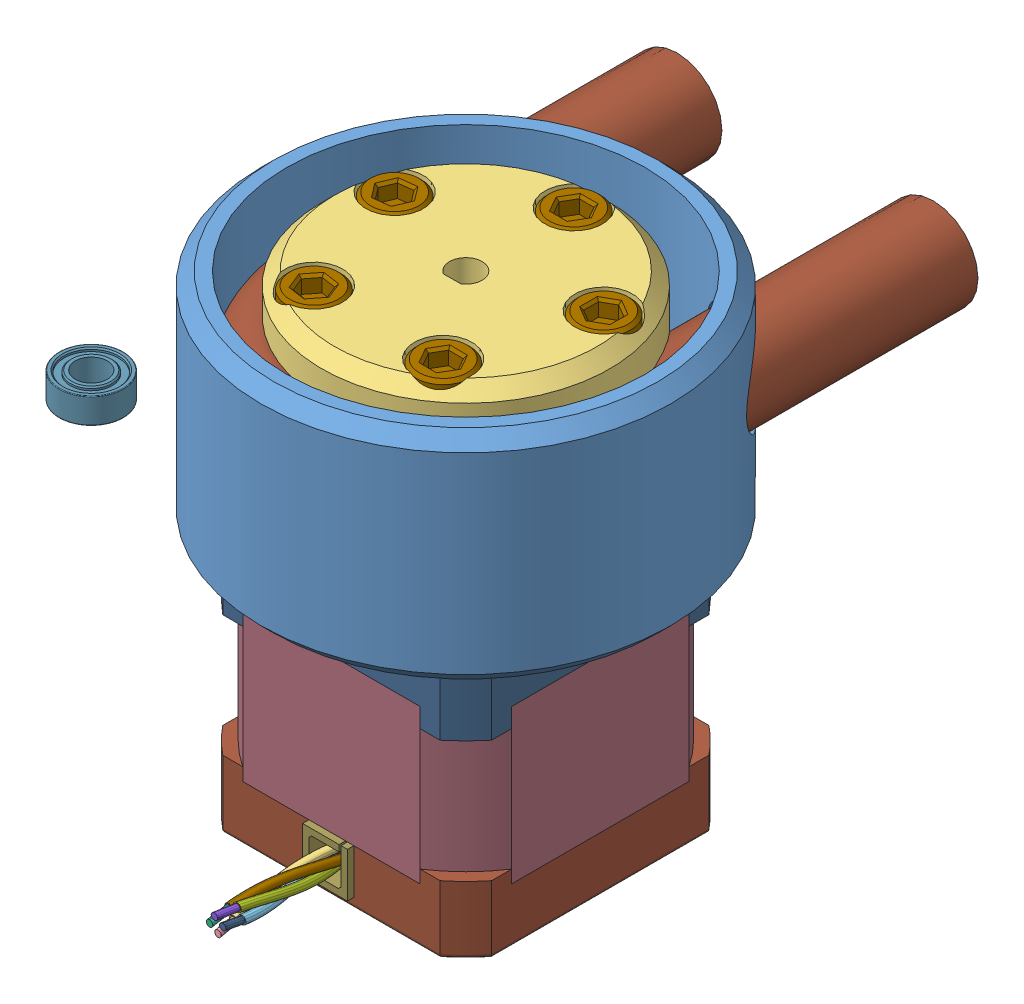
SolidWorks assembly pump, configuration Default. Lengths in mm.
Overall size (68.76 74.29 92).
175 component instances, 32 part files, 74 mates.
Components (placement in the parent):
- pump-shell-1: pump-shell [Default] at (23.8184 9.0777 41.5855) size (64 34 64)
- bottom-plate-1: bottom-plate [Default] at (23.8184 23.0777 41.5855) x (-0.999957 0 0.009262) z (0.009262 0 0.999957) size (52 18 52)
- top-plate-1: top-plate [Default] at (23.8184 35.0777 41.5855) x (-0.814427 0 -0.580267) z (0.580267 0 -0.814427) size (45 8.29 45)
- 625zz.STEP-1: 625zz.STEP [Default] at (23.8184 16.0777 41.5855) x (0 -1 0) z (-0.839089 0 -0.543994) size (5 16 16)
  - SKF 625 Inner Race^SKF 625.STEP-1: SKF 625 Inner Race^SKF 625.STEP [Default] at origin size (5 8.4 8.4)
  - SKF 625 Outer Race^SKF 625.STEP-1: SKF 625 Outer Race^SKF 625.STEP [Default] at origin size (5 16 16)
  - SKF 625 Ball^SKF 625.STEP-1: SKF 625 Ball^SKF 625.STEP [Default] at origin size (2.38 2.38 2.38)
  - SKF 625 Ball^SKF 625.STEP-2: SKF 625 Ball^SKF 625.STEP [Default] x (1 0 0) z (0 0.707107 0.707107) size (2.38 2.38 2.38)
  - SKF 625 Ball^SKF 625.STEP-3: SKF 625 Ball^SKF 625.STEP [Default] x (1 0 0) z (0 1 0) size (2.38 2.38 2.38)
  - SKF 625 Ball^SKF 625.STEP-4: SKF 625 Ball^SKF 625.STEP [Default] x (1 0 0) z (0 0.707107 -0.707107) size (2.38 2.38 2.38)
  - SKF 625 Ball^SKF 625.STEP-5: SKF 625 Ball^SKF 625.STEP [Default] x (1 0 0) z (0 0 -1) size (2.38 2.38 2.38)
  - SKF 625 Ball^SKF 625.STEP-6: SKF 625 Ball^SKF 625.STEP [Default] x (1 0 0) z (0 -0.707107 -0.707107) size (2.38 2.38 2.38)
  - SKF 625 Ball^SKF 625.STEP-7: SKF 625 Ball^SKF 625.STEP [Default] x (1 0 0) z (0 -1 0) size (2.38 2.38 2.38)
  - SKF 625 Ball^SKF 625.STEP-8: SKF 625 Ball^SKF 625.STEP [Default] x (1 0 0) z (0 -0.707107 0.707107) size (2.38 2.38 2.38)
  - SKF 625 Cage^SKF 625.STEP-1: SKF 625 Cage^SKF 625.STEP [Default] at (2.5 0 0) x (0 0 -1) z (1 0 0) size (12.17 12.17 2.88)
- m5-spacer-1: m5-spacer [Default] at (23.8184 16.0777 41.5855) x (-0.754389 0 0.656427) z (-0.656427 0 -0.754389) size (10 1 10)
- 625zz.STEP-2: 625zz.STEP [Default] at (7.5901 29.0777 36.4783) x (0 -1 0) z (0 0 1) size (5 16 16)
  - SKF 625 Inner Race^SKF 625.STEP-1: SKF 625 Inner Race^SKF 625.STEP [Default] at origin size (5 8.4 8.4)
  - SKF 625 Outer Race^SKF 625.STEP-1: SKF 625 Outer Race^SKF 625.STEP [Default] at origin size (5 16 16)
  - SKF 625 Ball^SKF 625.STEP-1: SKF 625 Ball^SKF 625.STEP [Default] at origin size (2.38 2.38 2.38)
  - SKF 625 Ball^SKF 625.STEP-2: SKF 625 Ball^SKF 625.STEP [Default] x (1 0 0) z (0 0.707107 0.707107) size (2.38 2.38 2.38)
  - SKF 625 Ball^SKF 625.STEP-3: SKF 625 Ball^SKF 625.STEP [Default] x (1 0 0) z (0 1 0) size (2.38 2.38 2.38)
  - SKF 625 Ball^SKF 625.STEP-4: SKF 625 Ball^SKF 625.STEP [Default] x (1 0 0) z (0 0.707107 -0.707107) size (2.38 2.38 2.38)
  - SKF 625 Ball^SKF 625.STEP-5: SKF 625 Ball^SKF 625.STEP [Default] x (1 0 0) z (0 0 -1) size (2.38 2.38 2.38)
  - SKF 625 Ball^SKF 625.STEP-6: SKF 625 Ball^SKF 625.STEP [Default] x (1 0 0) z (0 -0.707107 -0.707107) size (2.38 2.38 2.38)
  - SKF 625 Ball^SKF 625.STEP-7: SKF 625 Ball^SKF 625.STEP [Default] x (1 0 0) z (0 -1 0) size (2.38 2.38 2.38)
  - SKF 625 Ball^SKF 625.STEP-8: SKF 625 Ball^SKF 625.STEP [Default] x (1 0 0) z (0 -0.707107 0.707107) size (2.38 2.38 2.38)
  - SKF 625 Cage^SKF 625.STEP-1: SKF 625 Cage^SKF 625.STEP [Default] at (2.5 0 0) x (0 0 -1) z (1 0 0) size (12.17 12.17 2.88)
- 625zz.STEP-3: 625zz.STEP [Default] at (7.5901 34.0777 36.4783) x (0 -1 0) z (0.968021 0 0.25087) size (5 16 16)
  - SKF 625 Inner Race^SKF 625.STEP-1: SKF 625 Inner Race^SKF 625.STEP [Default] at origin size (5 8.4 8.4)
  - SKF 625 Outer Race^SKF 625.STEP-1: SKF 625 Outer Race^SKF 625.STEP [Default] at origin size (5 16 16)
  - SKF 625 Ball^SKF 625.STEP-1: SKF 625 Ball^SKF 625.STEP [Default] at origin size (2.38 2.38 2.38)
  - SKF 625 Ball^SKF 625.STEP-2: SKF 625 Ball^SKF 625.STEP [Default] x (1 0 0) z (0 0.707107 0.707107) size (2.38 2.38 2.38)
  - SKF 625 Ball^SKF 625.STEP-3: SKF 625 Ball^SKF 625.STEP [Default] x (1 0 0) z (0 1 0) size (2.38 2.38 2.38)
  - SKF 625 Ball^SKF 625.STEP-4: SKF 625 Ball^SKF 625.STEP [Default] x (1 0 0) z (0 0.707107 -0.707107) size (2.38 2.38 2.38)
  - SKF 625 Ball^SKF 625.STEP-5: SKF 625 Ball^SKF 625.STEP [Default] x (1 0 0) z (0 0 -1) size (2.38 2.38 2.38)
  - SKF 625 Ball^SKF 625.STEP-6: SKF 625 Ball^SKF 625.STEP [Default] x (1 0 0) z (0 -0.707107 -0.707107) size (2.38 2.38 2.38)
  - SKF 625 Ball^SKF 625.STEP-7: SKF 625 Ball^SKF 625.STEP [Default] x (1 0 0) z (0 -1 0) size (2.38 2.38 2.38)
  - SKF 625 Ball^SKF 625.STEP-8: SKF 625 Ball^SKF 625.STEP [Default] x (1 0 0) z (0 -0.707107 0.707107) size (2.38 2.38 2.38)
  - SKF 625 Cage^SKF 625.STEP-1: SKF 625 Cage^SKF 625.STEP [Default] at (2.5 0 0) x (0 0 -1) z (1 0 0) size (12.17 12.17 2.88)
- 625zz.STEP-4: 625zz.STEP [Default] at (33.9455 29.0777 55.2561) x (0 1 0) z (0 0 1) size (5 16 16)
  - SKF 625 Inner Race^SKF 625.STEP-1: SKF 625 Inner Race^SKF 625.STEP [Default] at origin size (5 8.4 8.4)
  - SKF 625 Outer Race^SKF 625.STEP-1: SKF 625 Outer Race^SKF 625.STEP [Default] at origin size (5 16 16)
  - SKF 625 Ball^SKF 625.STEP-1: SKF 625 Ball^SKF 625.STEP [Default] at origin size (2.38 2.38 2.38)
  - SKF 625 Ball^SKF 625.STEP-2: SKF 625 Ball^SKF 625.STEP [Default] x (1 0 0) z (0 0.707107 0.707107) size (2.38 2.38 2.38)
  - SKF 625 Ball^SKF 625.STEP-3: SKF 625 Ball^SKF 625.STEP [Default] x (1 0 0) z (0 1 0) size (2.38 2.38 2.38)
  - SKF 625 Ball^SKF 625.STEP-4: SKF 625 Ball^SKF 625.STEP [Default] x (1 0 0) z (0 0.707107 -0.707107) size (2.38 2.38 2.38)
  - SKF 625 Ball^SKF 625.STEP-5: SKF 625 Ball^SKF 625.STEP [Default] x (1 0 0) z (0 0 -1) size (2.38 2.38 2.38)
  - SKF 625 Ball^SKF 625.STEP-6: SKF 625 Ball^SKF 625.STEP [Default] x (1 0 0) z (0 -0.707107 -0.707107) size (2.38 2.38 2.38)
  - SKF 625 Ball^SKF 625.STEP-7: SKF 625 Ball^SKF 625.STEP [Default] x (1 0 0) z (0 -1 0) size (2.38 2.38 2.38)
  - SKF 625 Ball^SKF 625.STEP-8: SKF 625 Ball^SKF 625.STEP [Default] x (1 0 0) z (0 -0.707107 0.707107) size (2.38 2.38 2.38)
  - SKF 625 Cage^SKF 625.STEP-1: SKF 625 Cage^SKF 625.STEP [Default] at (2.5 0 0) x (0 0 -1) z (1 0 0) size (12.17 12.17 2.88)
- 625zz.STEP-5: 625zz.STEP [Default] at (33.9455 24.0777 55.2561) x (0 1 0) z (0.007155 0 0.999974) size (5 16 16)
  - SKF 625 Inner Race^SKF 625.STEP-1: SKF 625 Inner Race^SKF 625.STEP [Default] at origin size (5 8.4 8.4)
  - SKF 625 Outer Race^SKF 625.STEP-1: SKF 625 Outer Race^SKF 625.STEP [Default] at origin size (5 16 16)
  - SKF 625 Ball^SKF 625.STEP-1: SKF 625 Ball^SKF 625.STEP [Default] at origin size (2.38 2.38 2.38)
  - SKF 625 Ball^SKF 625.STEP-2: SKF 625 Ball^SKF 625.STEP [Default] x (1 0 0) z (0 0.707107 0.707107) size (2.38 2.38 2.38)
  - SKF 625 Ball^SKF 625.STEP-3: SKF 625 Ball^SKF 625.STEP [Default] x (1 0 0) z (0 1 0) size (2.38 2.38 2.38)
  - SKF 625 Ball^SKF 625.STEP-4: SKF 625 Ball^SKF 625.STEP [Default] x (1 0 0) z (0 0.707107 -0.707107) size (2.38 2.38 2.38)
  - SKF 625 Ball^SKF 625.STEP-5: SKF 625 Ball^SKF 625.STEP [Default] x (1 0 0) z (0 0 -1) size (2.38 2.38 2.38)
  - SKF 625 Ball^SKF 625.STEP-6: SKF 625 Ball^SKF 625.STEP [Default] x (1 0 0) z (0 -0.707107 -0.707107) size (2.38 2.38 2.38)
  - SKF 625 Ball^SKF 625.STEP-7: SKF 625 Ball^SKF 625.STEP [Default] x (1 0 0) z (0 -1 0) size (2.38 2.38 2.38)
  - SKF 625 Ball^SKF 625.STEP-8: SKF 625 Ball^SKF 625.STEP [Default] x (1 0 0) z (0 -0.707107 0.707107) size (2.38 2.38 2.38)
  - SKF 625 Cage^SKF 625.STEP-1: SKF 625 Cage^SKF 625.STEP [Default] at (2.5 0 0) x (0 0 -1) z (1 0 0) size (12.17 12.17 2.88)
- 625zz.STEP-6: 625zz.STEP [Default] at (13.9463 29.0777 55.4414) x (0 1 0) z (0.26967 0 0.962953) size (5 16 16)
  - SKF 625 Inner Race^SKF 625.STEP-1: SKF 625 Inner Race^SKF 625.STEP [Default] at origin size (5 8.4 8.4)
  - SKF 625 Outer Race^SKF 625.STEP-1: SKF 625 Outer Race^SKF 625.STEP [Default] at origin size (5 16 16)
  - SKF 625 Ball^SKF 625.STEP-1: SKF 625 Ball^SKF 625.STEP [Default] at origin size (2.38 2.38 2.38)
  - SKF 625 Ball^SKF 625.STEP-2: SKF 625 Ball^SKF 625.STEP [Default] x (1 0 0) z (0 0.707107 0.707107) size (2.38 2.38 2.38)
  - SKF 625 Ball^SKF 625.STEP-3: SKF 625 Ball^SKF 625.STEP [Default] x (1 0 0) z (0 1 0) size (2.38 2.38 2.38)
  - SKF 625 Ball^SKF 625.STEP-4: SKF 625 Ball^SKF 625.STEP [Default] x (1 0 0) z (0 0.707107 -0.707107) size (2.38 2.38 2.38)
  - SKF 625 Ball^SKF 625.STEP-5: SKF 625 Ball^SKF 625.STEP [Default] x (1 0 0) z (0 0 -1) size (2.38 2.38 2.38)
  - SKF 625 Ball^SKF 625.STEP-6: SKF 625 Ball^SKF 625.STEP [Default] x (1 0 0) z (0 -0.707107 -0.707107) size (2.38 2.38 2.38)
  - SKF 625 Ball^SKF 625.STEP-7: SKF 625 Ball^SKF 625.STEP [Default] x (1 0 0) z (0 -1 0) size (2.38 2.38 2.38)
  - SKF 625 Ball^SKF 625.STEP-8: SKF 625 Ball^SKF 625.STEP [Default] x (1 0 0) z (0 -0.707107 0.707107) size (2.38 2.38 2.38)
  - SKF 625 Cage^SKF 625.STEP-1: SKF 625 Cage^SKF 625.STEP [Default] at (2.5 0 0) x (0 0 -1) z (1 0 0) size (12.17 12.17 2.88)
- 625zz.STEP-7: 625zz.STEP [Default] at (13.9463 24.0777 55.4414) x (0 1 0) z (0.019727 0 0.999805) size (5 16 16)
  - SKF 625 Inner Race^SKF 625.STEP-1: SKF 625 Inner Race^SKF 625.STEP [Default] at origin size (5 8.4 8.4)
  - SKF 625 Outer Race^SKF 625.STEP-1: SKF 625 Outer Race^SKF 625.STEP [Default] at origin size (5 16 16)
  - SKF 625 Ball^SKF 625.STEP-1: SKF 625 Ball^SKF 625.STEP [Default] at origin size (2.38 2.38 2.38)
  - SKF 625 Ball^SKF 625.STEP-2: SKF 625 Ball^SKF 625.STEP [Default] x (1 0 0) z (0 0.707107 0.707107) size (2.38 2.38 2.38)
  - SKF 625 Ball^SKF 625.STEP-3: SKF 625 Ball^SKF 625.STEP [Default] x (1 0 0) z (0 1 0) size (2.38 2.38 2.38)
  - SKF 625 Ball^SKF 625.STEP-4: SKF 625 Ball^SKF 625.STEP [Default] x (1 0 0) z (0 0.707107 -0.707107) size (2.38 2.38 2.38)
  - SKF 625 Ball^SKF 625.STEP-5: SKF 625 Ball^SKF 625.STEP [Default] x (1 0 0) z (0 0 -1) size (2.38 2.38 2.38)
  - SKF 625 Ball^SKF 625.STEP-6: SKF 625 Ball^SKF 625.STEP [Default] x (1 0 0) z (0 -0.707107 -0.707107) size (2.38 2.38 2.38)
  - SKF 625 Ball^SKF 625.STEP-7: SKF 625 Ball^SKF 625.STEP [Default] x (1 0 0) z (0 -1 0) size (2.38 2.38 2.38)
  - SKF 625 Ball^SKF 625.STEP-8: SKF 625 Ball^SKF 625.STEP [Default] x (1 0 0) z (0 -0.707107 0.707107) size (2.38 2.38 2.38)
  - SKF 625 Cage^SKF 625.STEP-1: SKF 625 Cage^SKF 625.STEP [Default] at (2.5 0 0) x (0 0 -1) z (1 0 0) size (12.17 12.17 2.88)
- m5-spacer-2: m5-spacer [Default] at (13.9463 34.0777 55.4414) size (10 1 10)
- m5-spacer-3: m5-spacer [Default] at (13.9463 24.0777 55.4414) x (-0.837169 0 -0.546944) z (-0.546944 0 0.837169) size (10 1 10)
- m5-spacer-4: m5-spacer [Default] at (33.9455 24.0777 55.2561) x (-0.837169 0 -0.546944) z (-0.546944 0 0.837169) size (10 1 10)
- m5-spacer-5: m5-spacer [Default] at (39.9494 24.0777 36.1786) x (-0.837169 0 -0.546944) z (-0.546944 0 0.837169) size (10 1 10)
- m5-spacer-6: m5-spacer [Default] at (33.9455 34.0777 55.2561) size (10 1 10)
- m5-spacer-7: m5-spacer [Default] at (7.5901 34.0777 36.4783) x (-1 0 0) z (0 0 -1) size (10 1 10)
- m5-spacer-8: m5-spacer [Default] at (39.9494 34.0777 36.1786) x (-1 0 0) z (0 0 -1) size (10 1 10)
- m5-spacer-9: m5-spacer [Default] at (23.6609 34.0777 24.5732) x (-1 0 0) z (0 0 -1) size (10 1 10)
- m5-spacer-10: m5-spacer [Default] at (23.6609 24.0777 24.5732) x (-0.837169 0 -0.546944) z (-0.546944 0 0.837169) size (10 1 10)
- m5-spacer-11: m5-spacer [Default] at (7.5901 24.0777 36.4783) x (-0.837169 0 -0.546944) z (-0.546944 0 0.837169) size (10 1 10)
- 625zz.STEP-8: 625zz.STEP [Default] at (39.9494 34.0777 36.1786) x (0 -1 0) z (0.880718 0 0.47364) size (5 16 16)
  - SKF 625 Inner Race^SKF 625.STEP-1: SKF 625 Inner Race^SKF 625.STEP [Default] at origin size (5 8.4 8.4)
  - SKF 625 Outer Race^SKF 625.STEP-1: SKF 625 Outer Race^SKF 625.STEP [Default] at origin size (5 16 16)
  - SKF 625 Ball^SKF 625.STEP-1: SKF 625 Ball^SKF 625.STEP [Default] at origin size (2.38 2.38 2.38)
  - SKF 625 Ball^SKF 625.STEP-2: SKF 625 Ball^SKF 625.STEP [Default] x (1 0 0) z (0 0.707107 0.707107) size (2.38 2.38 2.38)
  - SKF 625 Ball^SKF 625.STEP-3: SKF 625 Ball^SKF 625.STEP [Default] x (1 0 0) z (0 1 0) size (2.38 2.38 2.38)
  - SKF 625 Ball^SKF 625.STEP-4: SKF 625 Ball^SKF 625.STEP [Default] x (1 0 0) z (0 0.707107 -0.707107) size (2.38 2.38 2.38)
  - SKF 625 Ball^SKF 625.STEP-5: SKF 625 Ball^SKF 625.STEP [Default] x (1 0 0) z (0 0 -1) size (2.38 2.38 2.38)
  - SKF 625 Ball^SKF 625.STEP-6: SKF 625 Ball^SKF 625.STEP [Default] x (1 0 0) z (0 -0.707107 -0.707107) size (2.38 2.38 2.38)
  - SKF 625 Ball^SKF 625.STEP-7: SKF 625 Ball^SKF 625.STEP [Default] x (1 0 0) z (0 -1 0) size (2.38 2.38 2.38)
  - SKF 625 Ball^SKF 625.STEP-8: SKF 625 Ball^SKF 625.STEP [Default] x (1 0 0) z (0 -0.707107 0.707107) size (2.38 2.38 2.38)
  - SKF 625 Cage^SKF 625.STEP-1: SKF 625 Cage^SKF 625.STEP [Default] at (2.5 0 0) x (0 0 -1) z (1 0 0) size (12.17 12.17 2.88)
- 625zz.STEP-9: 625zz.STEP [Default] at (39.9494 29.0777 36.1786) x (0 -1 0) z (0.968021 0 0.25087) size (5 16 16)
  - SKF 625 Inner Race^SKF 625.STEP-1: SKF 625 Inner Race^SKF 625.STEP [Default] at origin size (5 8.4 8.4)
  - SKF 625 Outer Race^SKF 625.STEP-1: SKF 625 Outer Race^SKF 625.STEP [Default] at origin size (5 16 16)
  - SKF 625 Ball^SKF 625.STEP-1: SKF 625 Ball^SKF 625.STEP [Default] at origin size (2.38 2.38 2.38)
  - SKF 625 Ball^SKF 625.STEP-2: SKF 625 Ball^SKF 625.STEP [Default] x (1 0 0) z (0 0.707107 0.707107) size (2.38 2.38 2.38)
  - SKF 625 Ball^SKF 625.STEP-3: SKF 625 Ball^SKF 625.STEP [Default] x (1 0 0) z (0 1 0) size (2.38 2.38 2.38)
  - SKF 625 Ball^SKF 625.STEP-4: SKF 625 Ball^SKF 625.STEP [Default] x (1 0 0) z (0 0.707107 -0.707107) size (2.38 2.38 2.38)
  - SKF 625 Ball^SKF 625.STEP-5: SKF 625 Ball^SKF 625.STEP [Default] x (1 0 0) z (0 0 -1) size (2.38 2.38 2.38)
  - SKF 625 Ball^SKF 625.STEP-6: SKF 625 Ball^SKF 625.STEP [Default] x (1 0 0) z (0 -0.707107 -0.707107) size (2.38 2.38 2.38)
  - SKF 625 Ball^SKF 625.STEP-7: SKF 625 Ball^SKF 625.STEP [Default] x (1 0 0) z (0 -1 0) size (2.38 2.38 2.38)
  - SKF 625 Ball^SKF 625.STEP-8: SKF 625 Ball^SKF 625.STEP [Default] x (1 0 0) z (0 -0.707107 0.707107) size (2.38 2.38 2.38)
  - SKF 625 Cage^SKF 625.STEP-1: SKF 625 Cage^SKF 625.STEP [Default] at (2.5 0 0) x (0 0 -1) z (1 0 0) size (12.17 12.17 2.88)
- 625zz.STEP-10: 625zz.STEP [Default] at (23.6609 34.0777 24.5732) x (0 -1 0) z (0.667894 0 -0.744257) size (5 16 16)
  - SKF 625 Inner Race^SKF 625.STEP-1: SKF 625 Inner Race^SKF 625.STEP [Default] at origin size (5 8.4 8.4)
  - SKF 625 Outer Race^SKF 625.STEP-1: SKF 625 Outer Race^SKF 625.STEP [Default] at origin size (5 16 16)
  - SKF 625 Ball^SKF 625.STEP-1: SKF 625 Ball^SKF 625.STEP [Default] at origin size (2.38 2.38 2.38)
  - SKF 625 Ball^SKF 625.STEP-2: SKF 625 Ball^SKF 625.STEP [Default] x (1 0 0) z (0 0.707107 0.707107) size (2.38 2.38 2.38)
  - SKF 625 Ball^SKF 625.STEP-3: SKF 625 Ball^SKF 625.STEP [Default] x (1 0 0) z (0 1 0) size (2.38 2.38 2.38)
  - SKF 625 Ball^SKF 625.STEP-4: SKF 625 Ball^SKF 625.STEP [Default] x (1 0 0) z (0 0.707107 -0.707107) size (2.38 2.38 2.38)
  - SKF 625 Ball^SKF 625.STEP-5: SKF 625 Ball^SKF 625.STEP [Default] x (1 0 0) z (0 0 -1) size (2.38 2.38 2.38)
  - SKF 625 Ball^SKF 625.STEP-6: SKF 625 Ball^SKF 625.STEP [Default] x (1 0 0) z (0 -0.707107 -0.707107) size (2.38 2.38 2.38)
  - SKF 625 Ball^SKF 625.STEP-7: SKF 625 Ball^SKF 625.STEP [Default] x (1 0 0) z (0 -1 0) size (2.38 2.38 2.38)
  - SKF 625 Ball^SKF 625.STEP-8: SKF 625 Ball^SKF 625.STEP [Default] x (1 0 0) z (0 -0.707107 0.707107) size (2.38 2.38 2.38)
  - SKF 625 Cage^SKF 625.STEP-1: SKF 625 Cage^SKF 625.STEP [Default] at (2.5 0 0) x (0 0 -1) z (1 0 0) size (12.17 12.17 2.88)
- 625zz.STEP-11: 625zz.STEP [Default] at (23.6609 29.0777 24.5732) x (0 -1 0) z (0.968021 0 0.25087) size (5 16 16)
  - SKF 625 Inner Race^SKF 625.STEP-1: SKF 625 Inner Race^SKF 625.STEP [Default] at origin size (5 8.4 8.4)
  - SKF 625 Outer Race^SKF 625.STEP-1: SKF 625 Outer Race^SKF 625.STEP [Default] at origin size (5 16 16)
  - SKF 625 Ball^SKF 625.STEP-1: SKF 625 Ball^SKF 625.STEP [Default] at origin size (2.38 2.38 2.38)
  - SKF 625 Ball^SKF 625.STEP-2: SKF 625 Ball^SKF 625.STEP [Default] x (1 0 0) z (0 0.707107 0.707107) size (2.38 2.38 2.38)
  - SKF 625 Ball^SKF 625.STEP-3: SKF 625 Ball^SKF 625.STEP [Default] x (1 0 0) z (0 1 0) size (2.38 2.38 2.38)
  - SKF 625 Ball^SKF 625.STEP-4: SKF 625 Ball^SKF 625.STEP [Default] x (1 0 0) z (0 0.707107 -0.707107) size (2.38 2.38 2.38)
  - SKF 625 Ball^SKF 625.STEP-5: SKF 625 Ball^SKF 625.STEP [Default] x (1 0 0) z (0 0 -1) size (2.38 2.38 2.38)
  - SKF 625 Ball^SKF 625.STEP-6: SKF 625 Ball^SKF 625.STEP [Default] x (1 0 0) z (0 -0.707107 -0.707107) size (2.38 2.38 2.38)
  - SKF 625 Ball^SKF 625.STEP-7: SKF 625 Ball^SKF 625.STEP [Default] x (1 0 0) z (0 -1 0) size (2.38 2.38 2.38)
  - SKF 625 Ball^SKF 625.STEP-8: SKF 625 Ball^SKF 625.STEP [Default] x (1 0 0) z (0 -0.707107 0.707107) size (2.38 2.38 2.38)
  - SKF 625 Cage^SKF 625.STEP-1: SKF 625 Cage^SKF 625.STEP [Default] at (2.5 0 0) x (0 0 -1) z (1 0 0) size (12.17 12.17 2.88)
- m5-socket-23-1: m5-socket-23 [Default] at (23.6609 43.0777 24.5732) x (0 -1 0) z (-0.50599 0 0.862539) size (28 8.5 8.5)
- m5-socket-23-2: m5-socket-23 [Default] at (39.9494 43.0777 36.1786) x (0 -1 0) z (-0.86182 0 -0.507214) size (28 8.5 8.5)
- m5-socket-23-3: m5-socket-23 [Default] at (33.9455 43.0777 55.2561) x (0 -1 0) z (-0.50599 0 0.862539) size (28 8.5 8.5)
- m5-socket-23-4: m5-socket-23 [Default] at (13.9463 43.0777 55.4414) x (0 -1 0) z (-0.617121 0 0.786868) size (28 8.5 8.5)
- m5-socket-23-5: m5-socket-23 [Default] at (7.5901 43.0777 36.4783) x (0 -1 0) z (0.992432 0 -0.122792) size (28 8.5 8.5)
- nema17-40mm.step-1: nema17-40mm.step [Default] at (23.8184 9.0777 41.5855) x (-1 0 0) z (0 0 1) size (42 64 60)
  - Frontplate.step-1: Frontplate.step [Default] at (0 10.5 0) size (42 12.5 42)
  - Backplate.step-1: Backplate.step [Default] at (0 40 0) size (42 10.5 42)
  - Connenctor.step-1: Connenctor.step [Default] at (0 31.5 22) size (7 7 7)
  - Housing.step-1: Housing.step [Default] at (0 7.5 0) size (42 24 42)
  - Bearing dummy.step-1: Bearing dummy.step [Default] at (0 4 0) size (22 7 22)
  - Bearing dummy 01.step-1: Bearing dummy 01.step [Default] at (0 35 0) size (22 7 22)
  - Core.step-1: Core.step [Default] at origin size (30 62.5 30)
  - M3x34-Screw.step-1: M3x34-Screw.step [Default] at (15.5 37.6 15.5) x (1 0 0) z (0 1 0) size (5.5 5.5 36)
  - M3x34-Screw001.step-1: M3x34-Screw001.step [Default] at (-15.5 37.6 15.5) x (1 0 0) z (0 1 0) size (5.5 5.5 36)
  - M3x34-Screw002.step-1: M3x34-Screw002.step [Default] at (-15.5 37.6 -15.5) x (1 0 0) z (0 1 0) size (5.5 5.5 36)
  - M3x34-Screw003.step-1: M3x34-Screw003.step [Default] at (15.5 37.6 -15.5) x (1 0 0) z (0 1 0) size (5.5 5.5 36)
  - Cable-1of4.step-1: Cable-1of4.step [Default] at (0 35 0) size (3.44 3.69 21)
  - Copper-1of4.step-1: Copper-1of4.step [Default] at (0 35 0) size (2.77 3.05 24)
  - Cable-2of4.step-1: Cable-2of4.step [Default] at (0 35 0) x (0 1 0) z (0 0 1) size (3.44 3.69 21)
  - Copper-4of4.step-1: Copper-4of4.step [Default] at (0 35 0) x (0 -1 0) z (0 0 1) size (2.77 3.05 24)
  - Cable-3of4.step-1: Cable-3of4.step [Default] at (0 35 0) x (-1 0 0) z (0 0 1) size (3.44 3.69 21)
  - Copper-3of4.step-1: Copper-3of4.step [Default] at (0 35 0) x (-1 0 0) z (0 0 1) size (2.77 3.05 24)
  - Cable-4of4.step-1: Cable-4of4.step [Default] at (0 35 0) x (0 -1 0) z (0 0 1) size (3.44 3.69 21)
  - Copper-2of4.step-1: Copper-2of4.step [Default] at (0 35 0) x (0 1 0) z (0 0 1) size (2.77 3.05 24)
- silicone-tube-1: silicone-tube [Default] at (23.8184 29.0777 43.5855) x (0 0 -1) z (0 1 0) size (83.5 54.86 16.16)
- m3-nut-1: m3-nut [Default] at (23.8661 29.0777 46.7353) x (0.955477 0.294934 -0.00885) z (0.009262 0 0.999957) size (5.8 5.57 2.34)
- m3-round-6-1: m3-round-6 [m3-10] at (23.8818 29.0777 48.4307) x (0.974551 -0.223985 -0.009027) z (-0.223976 -0.974593 0.002075) size (5.7 7.65 5.7)
- MR105ZZ-1: MR105ZZ [Default] at (-7.9398 25.1535 68.3374) size (10 4 10)
Mates (geometry in assembly coordinates):
- Concentric1: concentric anti-aligned: cylinder of pump-shell-1 through (23.8184 9.0777 41.5855) axis (0 1 0) radius 12.5; cylinder of 625zz.STEP-1/SKF 625 Outer Race^SKF 625.STEP-1 through (23.8184 11.3777 41.5855) axis (0 -1 0) radius 8
- Concentric2: concentric aligned: cylinder of 625zz.STEP-1/SKF 625 Inner Race^SKF 625.STEP-1 through (23.8184 11.3777 41.5855) axis (0 -1 0) radius 2.5; cylinder of m5-spacer-1 through (23.8184 17.0777 41.5855) axis (0 -1 0) radius 2.6
- Coincident2: coincident anti-aligned: plane of 625zz.STEP-1/SKF 625 Inner Race^SKF 625.STEP-1 through (21.5881 16.0777 45.0258) normal (0 1 0); plane of m5-spacer-1 through (23.8184 16.0777 41.5855) normal (0 -1 0)
- Coincident3: coincident anti-aligned: plane of bottom-plate-1 through (23.8184 17.0777 41.5855) normal (0 -1 0); plane of m5-spacer-1 through (23.8184 17.0777 41.5855) normal (0 1 0)
- Concentric3: concentric anti-aligned: cylinder of pump-shell-1 through (23.8184 43.0777 41.5855) axis (0 -1 0) radius 28; cylinder of bottom-plate-1 through (23.8184 17.0777 41.5855) axis (0 1 0) radius 26
- Coincident4: coincident anti-aligned: plane of bottom-plate-1 through (18.8824 35.0777 48.5134) normal (0 1 0); plane of top-plate-1 through (23.8184 35.0777 41.5855) normal (0 -1 0)
- Concentric5: concentric aligned: cylinder of bottom-plate-1 through (13.9463 17.0777 55.4414) axis (0 1 0) radius 2.65; cylinder of 625zz.STEP-7/SKF 625 Inner Race^SKF 625.STEP-1 through (13.9463 28.7777 55.4414) axis (0 1 0) radius 2.5
- Coincident7: coincident anti-aligned: plane of 625zz.STEP-6/SKF 625 Outer Race^SKF 625.STEP-1 through (6.5316 29.0777 57.5178) normal (0 -1 0); plane of 625zz.STEP-7/SKF 625 Outer Race^SKF 625.STEP-1 through (7.2976 29.0777 55.5725) normal (0 1 0)
- Concentric6: concentric aligned: cylinder of 625zz.STEP-6/SKF 625 Outer Race^SKF 625.STEP-1 through (13.9463 33.7777 55.4414) axis (0 1 0) radius 8; cylinder of 625zz.STEP-7/SKF 625 Outer Race^SKF 625.STEP-1 through (13.9463 28.7777 55.4414) axis (0 1 0) radius 8
- Coincident8: coincident anti-aligned: plane of top-plate-1 through (23.8184 35.0777 41.5855) normal (0 -1 0); plane of m5-spacer-2 through (13.9463 35.0777 55.4414) normal (0 1 0)
- Concentric7: concentric anti-aligned: cylinder of 625zz.STEP-6/SKF 625 Outer Race^SKF 625.STEP-1 through (13.9463 33.7777 55.4414) axis (0 1 0) radius 8; cylinder of m5-spacer-2 through (13.9463 35.0777 55.4414) axis (0 -1 0) radius 5
- Coincident9: coincident anti-aligned: plane of bottom-plate-1 through (23.8184 23.0777 41.5855) normal (0 1 0); plane of m5-spacer-3 through (13.9463 23.0777 55.4414) normal (0 -1 0)
- Concentric8: concentric aligned: cylinder of 625zz.STEP-7/SKF 625 Outer Race^SKF 625.STEP-1 through (13.9463 28.7777 55.4414) axis (0 1 0) radius 8; cylinder of m5-spacer-3 through (13.9463 23.0777 55.4414) axis (0 1 0) radius 5
- Coincident10: coincident anti-aligned: plane of bottom-plate-1 through (23.8184 23.0777 41.5855) normal (0 1 0); plane of m5-spacer-4 through (33.9455 23.0777 55.2561) normal (0 -1 0)
- Concentric9: concentric aligned: cylinder of bottom-plate-1 through (33.9455 17.0777 55.2561) axis (0 1 0) radius 2.65; cylinder of m5-spacer-4 through (33.9455 23.0777 55.2561) axis (0 1 0) radius 2.6
- Coincident11: coincident anti-aligned: plane of 625zz.STEP-5/SKF 625 Outer Race^SKF 625.STEP-1 through (26.2457 24.0777 55.3112) normal (0 -1 0); plane of m5-spacer-4 through (33.9455 24.0777 55.2561) normal (0 1 0)
- Concentric10: concentric aligned: cylinder of bottom-plate-1 through (33.9455 17.0777 55.2561) axis (0 1 0) radius 2.65; cylinder of 625zz.STEP-5/SKF 625 Outer Race^SKF 625.STEP-1 through (33.9455 28.7777 55.2561) axis (0 1 0) radius 8
- Coincident12: coincident anti-aligned: plane of 625zz.STEP-4/SKF 625 Outer Race^SKF 625.STEP-1 through (26.2455 29.0777 55.2561) normal (0 -1 0); plane of 625zz.STEP-5/SKF 625 Outer Race^SKF 625.STEP-1 through (27.2957 29.0777 55.3037) normal (0 1 0)
- Concentric11: concentric aligned: cylinder of 625zz.STEP-4/SKF 625 Outer Race^SKF 625.STEP-1 through (33.9455 33.7777 55.2561) axis (0 1 0) radius 8; cylinder of 625zz.STEP-5/SKF 625 Outer Race^SKF 625.STEP-1 through (33.9455 28.7777 55.2561) axis (0 1 0) radius 8
- Coincident13: coincident anti-aligned: plane of top-plate-1 through (23.8184 35.0777 41.5855) normal (0 -1 0); plane of m5-spacer-6 through (33.9455 35.0777 55.2561) normal (0 1 0)
- Concentric12: concentric anti-aligned: cylinder of 625zz.STEP-4/SKF 625 Inner Race^SKF 625.STEP-1 through (33.9455 33.7777 55.2561) axis (0 1 0) radius 2.5; cylinder of m5-spacer-6 through (33.9455 35.0777 55.2561) axis (0 -1 0) radius 2.6
- Coincident14: coincident anti-aligned: plane of bottom-plate-1 through (23.8184 23.0777 41.5855) normal (0 1 0); plane of m5-spacer-5 through (39.9494 23.0777 36.1786) normal (0 -1 0)
- Concentric14: concentric aligned: cylinder of bottom-plate-1 through (39.9494 17.0777 36.1786) axis (0 1 0) radius 2.65; cylinder of m5-spacer-5 through (39.9494 23.0777 36.1786) axis (0 1 0) radius 2.6
- Concentric15: concentric aligned: cylinder of bottom-plate-1 through (23.6609 17.0777 24.5732) axis (0 1 0) radius 2.65; cylinder of m5-spacer-10 through (23.6609 23.0777 24.5732) axis (0 1 0) radius 2.6
- Coincident15: coincident anti-aligned: plane of bottom-plate-1 through (23.8184 23.0777 41.5855) normal (0 1 0); plane of m5-spacer-10 through (23.6609 23.0777 24.5732) normal (0 -1 0)
- Coincident16: coincident anti-aligned: plane of bottom-plate-1 through (23.8184 23.0777 41.5855) normal (0 1 0); plane of m5-spacer-11 through (7.5901 23.0777 36.4783) normal (0 -1 0)
- Concentric16: concentric aligned: cylinder of bottom-plate-1 through (7.5901 17.0777 36.4783) axis (0 1 0) radius 2.65; cylinder of m5-spacer-11 through (7.5901 23.0777 36.4783) axis (0 1 0) radius 2.6
- Coincident17: coincident anti-aligned: plane of 625zz.STEP-2/SKF 625 Inner Race^SKF 625.STEP-1 through (10.3901 24.0777 36.4783) normal (0 -1 0); plane of m5-spacer-11 through (7.5901 24.0777 36.4783) normal (0 1 0)
- Concentric17: concentric anti-aligned: cylinder of bottom-plate-1 through (7.5901 17.0777 36.4783) axis (0 1 0) radius 2.65; cylinder of 625zz.STEP-2/SKF 625 Outer Race^SKF 625.STEP-1 through (7.5901 24.3777 36.4783) axis (0 -1 0) radius 8
- Coincident18: coincident anti-aligned: plane of 625zz.STEP-2/SKF 625 Outer Race^SKF 625.STEP-1 through (15.2901 29.0777 36.4783) normal (0 1 0); plane of 625zz.STEP-3/SKF 625 Outer Race^SKF 625.STEP-1 through (9.2584 29.0777 30.041) normal (0 -1 0)
- Concentric18: concentric aligned: cylinder of 625zz.STEP-2/SKF 625 Outer Race^SKF 625.STEP-1 through (7.5901 24.3777 36.4783) axis (0 -1 0) radius 8; cylinder of 625zz.STEP-3/SKF 625 Outer Race^SKF 625.STEP-1 through (7.5901 29.3777 36.4783) axis (0 -1 0) radius 8
- Coincident19: coincident anti-aligned: plane of 625zz.STEP-3/SKF 625 Outer Race^SKF 625.STEP-1 through (9.5218 34.0777 29.0245) normal (0 1 0); plane of m5-spacer-7 through (7.5901 34.0777 36.4783) normal (0 -1 0)
- Concentric19: concentric aligned: cylinder of 625zz.STEP-3/SKF 625 Inner Race^SKF 625.STEP-1 through (7.5901 29.3777 36.4783) axis (0 -1 0) radius 2.5; cylinder of m5-spacer-7 through (7.5901 35.0777 36.4783) axis (0 -1 0) radius 5
- Coincident20: coincident anti-aligned: plane of m5-spacer-5 through (39.9494 24.0777 36.1786) normal (0 1 0); plane of 625zz.STEP-9/SKF 625 Inner Race^SKF 625.STEP-1 through (40.6518 24.0777 33.4681) normal (0 -1 0)
- Concentric20: concentric anti-aligned: cylinder of bottom-plate-1 through (39.9494 17.0777 36.1786) axis (0 1 0) radius 2.65; cylinder of 625zz.STEP-9/SKF 625 Outer Race^SKF 625.STEP-1 through (39.9494 24.3777 36.1786) axis (0 -1 0) radius 8
- Concentric21: concentric aligned: cylinder of 625zz.STEP-8/SKF 625 Outer Race^SKF 625.STEP-1 through (39.9494 29.3777 36.1786) axis (0 -1 0) radius 8; cylinder of 625zz.STEP-9/SKF 625 Outer Race^SKF 625.STEP-1 through (39.9494 24.3777 36.1786) axis (0 -1 0) radius 8
- Coincident21: coincident anti-aligned: plane of 625zz.STEP-8/SKF 625 Outer Race^SKF 625.STEP-1 through (43.0991 29.0777 30.3218) normal (0 -1 0); plane of 625zz.STEP-9/SKF 625 Outer Race^SKF 625.STEP-1 through (41.8811 29.0777 28.7248) normal (0 1 0)
- Coincident22: coincident anti-aligned: plane of m5-spacer-8 through (39.9494 34.0777 36.1786) normal (0 -1 0); plane of 625zz.STEP-8/SKF 625 Inner Race^SKF 625.STEP-1 through (41.8913 34.0777 32.5676) normal (0 1 0)
- Concentric22: concentric aligned: cylinder of m5-spacer-8 through (39.9494 35.0777 36.1786) axis (0 -1 0) radius 5; cylinder of 625zz.STEP-8/SKF 625 Inner Race^SKF 625.STEP-1 through (39.9494 29.3777 36.1786) axis (0 -1 0) radius 2.5
- Coincident23: coincident anti-aligned: plane of top-plate-1 through (23.8184 35.0777 41.5855) normal (0 -1 0); plane of m5-spacer-9 through (23.6609 35.0777 24.5732) normal (0 1 0)
- Concentric23: concentric anti-aligned: cylinder of m5-spacer-9 through (23.6609 35.0777 24.5732) axis (0 -1 0) radius 2.6; cylinder of m5-spacer-10 through (23.6609 23.0777 24.5732) axis (0 1 0) radius 2.6
- Concentric24: concentric anti-aligned: cylinder of bottom-plate-1 through (23.6609 17.0777 24.5732) axis (0 1 0) radius 2.65; cylinder of 625zz.STEP-11/SKF 625 Outer Race^SKF 625.STEP-1 through (23.6609 24.3777 24.5732) axis (0 -1 0) radius 8
- Coincident24: coincident anti-aligned: plane of m5-spacer-10 through (23.6609 24.0777 24.5732) normal (0 1 0); plane of 625zz.STEP-11/SKF 625 Outer Race^SKF 625.STEP-1 through (25.3291 24.0777 18.1359) normal (0 -1 0)
- Concentric25: concentric aligned: cylinder of 625zz.STEP-10/SKF 625 Outer Race^SKF 625.STEP-1 through (23.6609 29.3777 24.5732) axis (0 -1 0) radius 8; cylinder of 625zz.STEP-11/SKF 625 Outer Race^SKF 625.STEP-1 through (23.6609 24.3777 24.5732) axis (0 -1 0) radius 8
- Coincident25: coincident anti-aligned: plane of 625zz.STEP-10/SKF 625 Outer Race^SKF 625.STEP-1 through (18.7115 29.0777 20.1317) normal (0 -1 0); plane of 625zz.STEP-11/SKF 625 Outer Race^SKF 625.STEP-1 through (25.5926 29.0777 17.1195) normal (0 1 0)
- Concentric30: concentric anti-aligned: cylinder of bottom-plate-1 through (23.8184 17.0777 41.5855) axis (0 1 0) radius 26; cylinder of top-plate-1 through (23.8184 43.0777 41.5855) axis (0 -1 0) radius 22.5
- Coincident31: coincident anti-aligned: plane of top-plate-1 through (23.6609 38.0777 24.5732) normal (0 1 0); plane of m5-socket-23-1 through (25.8069 38.0777 25.8321) normal (0 -1 0)
- Concentric36: concentric anti-aligned: cylinder of top-plate-1 through (23.6609 43.0777 24.5732) axis (0 -1 0) radius 2.65; cylinder of m5-socket-23-1 through (23.6609 131.7832 24.5732) axis (0 1 0) radius 2.488
- Concentric37: concentric anti-aligned: cylinder of top-plate-1 through (39.9494 43.0777 36.1786) axis (0 -1 0) radius 2.65; cylinder of m5-socket-23-2 through (39.9494 131.7832 36.1786) axis (0 1 0) radius 2.488
- Coincident32: coincident anti-aligned: plane of top-plate-1 through (39.9494 38.0777 36.1786) normal (0 1 0); plane of m5-socket-23-2 through (38.6874 38.0777 38.3228) normal (0 -1 0)
- Concentric38: concentric anti-aligned: cylinder of top-plate-1 through (33.9455 43.0777 55.2561) axis (0 -1 0) radius 2.65; cylinder of m5-socket-23-3 through (33.9455 131.7832 55.2561) axis (0 1 0) radius 2.488
- Coincident33: coincident anti-aligned: plane of top-plate-1 through (33.9455 38.0777 55.2561) normal (0 1 0); plane of m5-socket-23-3 through (36.0915 38.0777 56.515) normal (0 -1 0)
- Concentric39: concentric anti-aligned: cylinder of top-plate-1 through (13.9463 43.0777 55.4414) axis (0 -1 0) radius 2.65; cylinder of m5-socket-23-4 through (13.9463 131.7832 55.4414) axis (0 1 0) radius 2.488
- Coincident34: coincident anti-aligned: plane of top-plate-1 through (13.9463 38.0777 55.4414) normal (0 1 0); plane of m5-socket-23-4 through (15.9041 38.0777 56.9768) normal (0 -1 0)
- Concentric40: concentric anti-aligned: cylinder of top-plate-1 through (7.5901 43.0777 36.4783) axis (0 -1 0) radius 2.65; cylinder of m5-socket-23-5 through (7.5901 131.7832 36.4783) axis (0 1 0) radius 2.488
- Coincident35: coincident anti-aligned: plane of top-plate-1 through (7.5901 38.0777 36.4783) normal (0 1 0); plane of m5-socket-23-5 through (7.2846 38.0777 34.0091) normal (0 -1 0)
- Concentric41: concentric aligned: cylinder of bottom-plate-1 through (13.9463 17.0777 55.4414) axis (0 1 0) radius 2.65; cylinder of m5-socket-23-4 through (13.9463 131.7832 55.4414) axis (0 1 0) radius 2.488
- Coincident36: coincident anti-aligned: plane of pump-shell-1 through (23.8184 9.0777 41.5855) normal (0 -1 0); plane of nema17-40mm.step-1/Frontplate.step-1 through (23.8184 9.0777 41.5855) normal (0 1 0)
- Concentric42: concentric anti-aligned: cylinder of pump-shell-1 through (39.3184 9.0777 57.0855) axis (0 1 0) radius 1.75; cylinder of nema17-40mm.step-1/Frontplate.step-1 through (39.3184 -1.4223 57.0855) axis (0 -1 0) radius 1.23
- Concentric43: concentric anti-aligned: cylinder of pump-shell-1 through (8.3184 9.0777 57.0855) axis (0 1 0) radius 1.75; cylinder of nema17-40mm.step-1/Frontplate.step-1 through (8.3184 -1.4223 57.0855) axis (0 -1 0) radius 1.23
- Concentric44: concentric anti-aligned: cylinder of bottom-plate-1 through (24.0593 29.0777 67.5844) axis (-0.009262 0 -0.999957) radius 1.75; cylinder of m3-heatset-large-1 through (19.7818 34.0777 38.7206) axis (-0.815485 0 -0.578778) radius 2.125
- Coincident37: coincident aligned: plane of bottom-plate-1 through (25.2094 17.0777 43.7227) normal (-0.009262 0 -0.999957); plane of m3-heatset-large-1 through (21.8571 35.4337 40.9799) normal (0.815485 0 0.578778)
- Concentric45: concentric aligned: cylinder of pump-shell-1 through (3.8184 29.0777 9.5855) axis (0 0 1) radius 7.5; cylinder of silicone-tube-1 through (3.8184 29.0777 -11.4145) axis (0 0 1) radius 7
- Concentric46: concentric aligned: cylinder of pump-shell-1 through (43.8184 29.0777 9.5855) axis (0 0 1) radius 7.5; cylinder of silicone-tube-1 through (43.8184 29.0777 -11.4145) axis (0 0 1) radius 7
- Distance1: distance = 53 mm anti-aligned: plane of silicone-tube-1 through (43.8184 29.0777 -11.4145) normal (0 0 -1); plane of nema17-40mm.step-1 through (23.8184 9.0777 41.5855) normal (0 0 1)
- Coincident39: coincident anti-aligned: plane of bottom-plate-1 through (26.9567 25.0777 45.7066) normal (0.009262 0 0.999957); plane of m3-nut-1 through (23.8569 29.0777 45.7353) normal (-0.009262 0 -0.999957)
- Concentric47: concentric anti-aligned: cylinder of bottom-plate-1 through (24.0593 29.0777 67.5844) axis (-0.009262 0 -0.999957) radius 1.75; circle of m3-nut-1
- Parallel3: parallel aligned: plane of bottom-plate-1 through (23.8184 25.0777 41.5855) normal (0 1 0); plane of m3-nut-1 through (25.2503 31.4592 47.7225) normal (0 1 0)
- Concentric48: concentric anti-aligned: cylinder of bottom-plate-1 through (24.0593 29.0777 67.5844) axis (-0.009262 0 -0.999957) radius 1.75; cylinder of m3-socket-6-1 through (-73.6997 34.0777 62.3557) axis (-0.978062 0 0.208315) radius 1.49
- Coincident41: coincident anti-aligned: plane of bottom-plate-1 through (23.8879 29.0777 49.0852) normal (0.009262 0 0.999957); plane of m3-socket-6-1 through (15.7063 33.5172 41.9017) normal (0.978062 0 -0.208315)
- Concentric49: concentric aligned: cylinder of bottom-plate-1 through (24.0593 29.0777 67.5844) axis (-0.009262 0 -0.999957) radius 1.75; cylinder of m3-round-6-1 through (23.8818 29.0777 48.4307) axis (-0.009262 0 -0.999957) radius 1.5
- Coincident42: coincident anti-aligned: plane of bottom-plate-1 through (23.8879 29.0777 49.0852) normal (0.009262 0 0.999957); plane of m3-round-6-1 through (21.1104 29.716 49.1109) normal (-0.009262 0 -0.999957)
- Coincident43: coincident anti-aligned: plane of 625zz.STEP-7/SKF 625 Inner Race^SKF 625.STEP-1 through (9.8471 24.0777 55.5222) normal (0 -1 0); plane of m5-spacer-3 through (13.9463 24.0777 55.4414) normal (0 1 0)
- Coincident44: coincident anti-aligned: plane of 625zz.STEP-1/SKF 625 Inner Race^SKF 625.STEP-1 through (22.2953 11.0777 43.935) normal (0 -1 0); plane of nema17-40mm.step-1/Frontplate.step-1 through (23.8184 11.0777 41.5855) normal (0 1 0)
